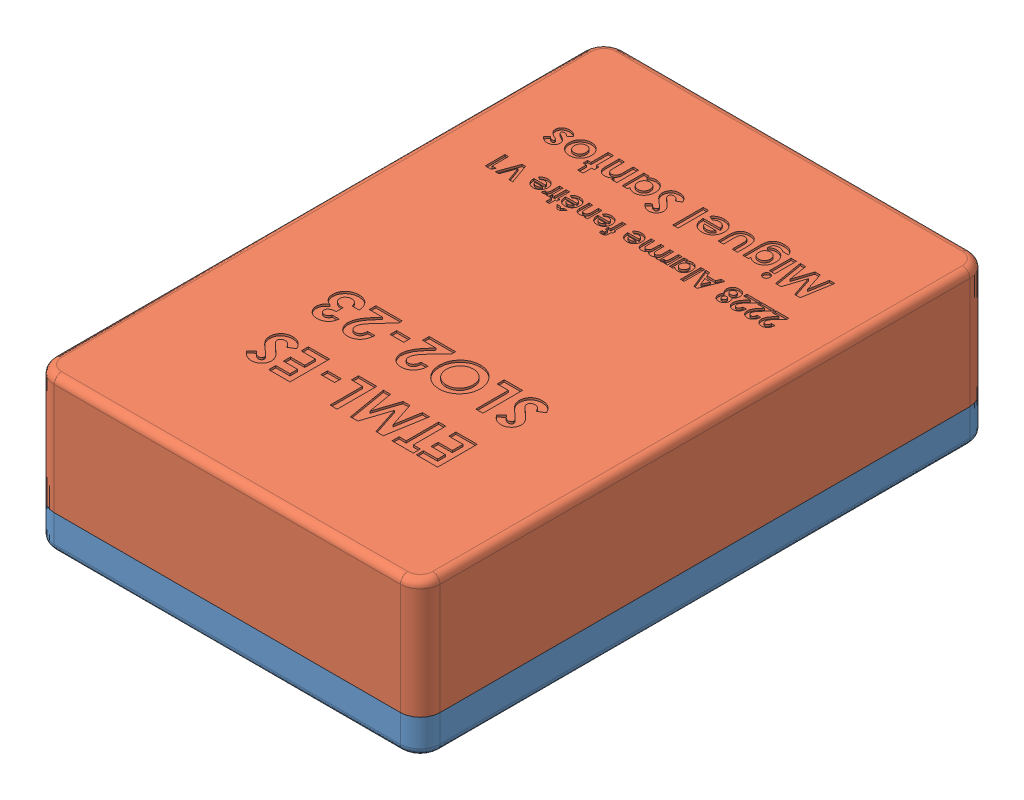
SolidWorks assembly 2228_Emetteur_Assembly, configuration Défaut. Lengths in mm.
Overall size (78 31 115.1).
221 component instances, 55 part files, 8 mates.
Components (placement in the parent):
- 2228_Emetteur_Bottom-1: 2228_Emetteur_Bottom [Défaut] at origin size (78 8.5 115.1)
- 2228_Emetteur_Top-1: 2228_Emetteur_Top [Défaut] at (0 31 0) x (-1 0 0) z (0 0 1) size (78 28 115.1)
- 22280A_AlarmeFenetre_Emetteur.step-1: 22280A_AlarmeFenetre_Emetteur.step [Défaut] at (30 7.1063 -64.5) x (-1 0 0) z (0 1 0) size (64.32 60 20.1)
  - Board.step-1: Board.step [Défaut] at origin size (60 60 1.61)
    - Open CASCADE STEP translator 6.8 1.1.1.step-1: Open CASCADE STEP translator 6.8 1.1.1.step [Défaut] at (0 0 -1.6063) size (60 60 1.61)
  - X3.step-1: X3.step [Défaut] at origin size (5.08 5.08 11.54)
    - 61300421121.step-1: 61300421121.step [Défaut] at (31.75 25 1.27) x (0 1 0) z (1 0 0) size (5.08 11.54 5.08)
      - Open CASCADE STEP translator 6.8 1.2.1.1.step-1: Open CASCADE STEP translator 6.8 1.2.1.1.step [Défaut] at origin size (5.08 2.54 5.08)
      - Open CASCADE STEP translator 6.8 1.2.1.2.step-1: Open CASCADE STEP translator 6.8 1.2.1.2.step [Défaut] at origin size (0.64 11.54 0.64)
      - Open CASCADE STEP translator 6.8 1.2.1.3.step-1: Open CASCADE STEP translator 6.8 1.2.1.3.step [Défaut] at origin size (0.64 11.54 0.64)
      - Open CASCADE STEP translator 6.8 1.2.1.4.step-1: Open CASCADE STEP translator 6.8 1.2.1.4.step [Défaut] at origin size (0.64 11.54 0.64)
      - Open CASCADE STEP translator 6.8 1.2.1.5.step-1: Open CASCADE STEP translator 6.8 1.2.1.5.step [Défaut] at origin size (0.64 11.54 0.64)
  - X5.step-1: X5.step [Défaut] at origin size (5.08 5.08 11.54)
    - 61300421121.step-1: 61300421121.step [Défaut] at (21.59 25 1.27) x (0 1 0) z (1 0 0) size (5.08 11.54 5.08)
      - Open CASCADE STEP translator 6.8 1.2.1.1.step-1: Open CASCADE STEP translator 6.8 1.2.1.1.step [Défaut] at origin size (5.08 2.54 5.08)
      - Open CASCADE STEP translator 6.8 1.2.1.2.step-1: Open CASCADE STEP translator 6.8 1.2.1.2.step [Défaut] at origin size (0.64 11.54 0.64)
      - Open CASCADE STEP translator 6.8 1.2.1.3.step-1: Open CASCADE STEP translator 6.8 1.2.1.3.step [Défaut] at origin size (0.64 11.54 0.64)
      - Open CASCADE STEP translator 6.8 1.2.1.4.step-1: Open CASCADE STEP translator 6.8 1.2.1.4.step [Défaut] at origin size (0.64 11.54 0.64)
      - Open CASCADE STEP translator 6.8 1.2.1.5.step-1: Open CASCADE STEP translator 6.8 1.2.1.5.step [Défaut] at origin size (0.64 11.54 0.64)
  - X4.step-1: X4.step [Défaut] at origin size (5.08 5.08 11.54)
    - 61300421121.step-1: 61300421121.step [Défaut] at (10.16 26.27 1.27) x (-1 0 0) z (0 1 0) size (5.08 11.54 5.08)
      - Open CASCADE STEP translator 6.8 1.2.1.1.step-1: Open CASCADE STEP translator 6.8 1.2.1.1.step [Défaut] at origin size (5.08 2.54 5.08)
      - Open CASCADE STEP translator 6.8 1.2.1.2.step-1: Open CASCADE STEP translator 6.8 1.2.1.2.step [Défaut] at origin size (0.64 11.54 0.64)
      - Open CASCADE STEP translator 6.8 1.2.1.3.step-1: Open CASCADE STEP translator 6.8 1.2.1.3.step [Défaut] at origin size (0.64 11.54 0.64)
      - Open CASCADE STEP translator 6.8 1.2.1.4.step-1: Open CASCADE STEP translator 6.8 1.2.1.4.step [Défaut] at origin size (0.64 11.54 0.64)
      - Open CASCADE STEP translator 6.8 1.2.1.5.step-1: Open CASCADE STEP translator 6.8 1.2.1.5.step [Défaut] at origin size (0.64 11.54 0.64)
  - X2.step-1: X2.step [Défaut] at origin size (5.08 5.08 11.54)
    - 61300421121.step-1: 61300421121.step [Défaut] at (39.37 25 1.27) x (0 -1 0) z (-1 0 0) size (5.08 11.54 5.08)
      - Open CASCADE STEP translator 6.8 1.2.1.1.step-1: Open CASCADE STEP translator 6.8 1.2.1.1.step [Défaut] at origin size (5.08 2.54 5.08)
      - Open CASCADE STEP translator 6.8 1.2.1.2.step-1: Open CASCADE STEP translator 6.8 1.2.1.2.step [Défaut] at origin size (0.64 11.54 0.64)
      - Open CASCADE STEP translator 6.8 1.2.1.3.step-1: Open CASCADE STEP translator 6.8 1.2.1.3.step [Défaut] at origin size (0.64 11.54 0.64)
      - Open CASCADE STEP translator 6.8 1.2.1.4.step-1: Open CASCADE STEP translator 6.8 1.2.1.4.step [Défaut] at origin size (0.64 11.54 0.64)
      - Open CASCADE STEP translator 6.8 1.2.1.5.step-1: Open CASCADE STEP translator 6.8 1.2.1.5.step [Défaut] at origin size (0.64 11.54 0.64)
  - X1.step-1: X1.step [Défaut] at origin size (2.54 5.08 11.54)
    - STEP-61300211121-rev1.step-1: STEP-61300211121-rev1.step [Défaut] at (11.9999 6.27 1.27) x (0 -1 0) z (-1 0 0) size (5.08 11.54 2.54)
      - 6130xx11121_PIN.step-1: 6130xx11121_PIN.step [Défaut] at (-1.27 1.5 0) x (1 0 0) z (0 -1 0) size (0.64 0.64 11.54)
      - 6130xx11121_PIN.step-2: 6130xx11121_PIN.step [Défaut] at (1.27 1.5 0) x (1 0 0) z (0 -1 0) size (0.64 0.64 11.54)
      - 61300211121.step-1: 61300211121.step [Défaut] at origin size (5.08 2.54 2.54)
  - VSTOR.step-1: VSTOR.step [Défaut] at origin size (3.81 2.03 2.29)
    - keystone-PN5019.step-1: keystone-PN5019.step [Défaut] at (56.9999 22.0009 0) x (1 0 0) z (0 -1 0) size (3.81 2.29 2.03)
  - VSEC.step-1: VSEC.step [Défaut] at origin size (3.81 2.03 2.29)
    - keystone-PN5019.step-1: keystone-PN5019.step [Défaut] at (57.0001 15.9991 0) x (-1 0 0) z (0 1 0) size (3.81 2.29 2.03)
  - VMUL.step-1: VMUL.step [Défaut] at origin size (3.81 2.03 2.29)
    - keystone-PN5019.step-1: keystone-PN5019.step [Défaut] at (3.0001 21.9991 0) x (-1 0 0) z (0 1 0) size (3.81 2.29 2.03)
  - VIN.step-1: VIN.step [Défaut] at origin size (3.81 2.03 2.29)
    - keystone-PN5019.step-1: keystone-PN5019.step [Défaut] at (2.9999 10.0009 0) x (1 0 0) z (0 -1 0) size (3.81 2.29 2.03)
  - VCC.step-1: VCC.step [Défaut] at origin size (3.81 2.03 2.29)
    - keystone-PN5019.step-1: keystone-PN5019.step [Défaut] at (3.0001 27.9991 0) x (-1 0 0) z (0 1 0) size (3.81 2.29 2.03)
  - U6.step-1: U6.step [Défaut] at origin size (46.04 19.26 18.6)
    - 61301011821.step-1: 61301011821.step [Défaut] at (1.27 49.62 0) x (1 0 0) z (0 0 1) size (25.9 2.5 11.6)
      - Body.step-1: Body.step [Défaut] at origin size (25.9 2.5 8.5)
      - LeadsArray.step-1: LeadsArray.step [Défaut] at origin size (23.46 0.6 4.8)
    - 61301011821.step-2: 61301011821.step [Défaut] at (1.27 34.38 0) x (1 0 0) z (0 0 1) size (25.9 2.5 11.6)
      - Body.step-1: Body.step [Défaut] at origin size (25.9 2.5 8.5)
      - LeadsArray.step-1: LeadsArray.step [Défaut] at origin size (23.46 0.6 4.8)
    - Conn_Wurth_Elektronik_61301011121_eec.step-1: Conn_Wurth_Elektronik_61301011121_eec.step [Défaut] at (12.7 49.62 10) x (1 0 0) z (0 1 0) size (25.4 11.74 4.02)
      - Package.step-1: Package.step [Défaut] at origin size (25.4 2.54 2.54)
      - Pins.step-1: Pins.step [Défaut] at origin size (23.5 11.74 0.64)
      - Logo.step-1: Logo.step [Défaut] at (12.7 -1.27 1.27) size (5.18 4.49 4.02)
    - Conn_Wurth_Elektronik_61301011121_eec.step-2: Conn_Wurth_Elektronik_61301011121_eec.step [Défaut] at (12.7 34.38 10) x (1 0 0) z (0 1 0) size (25.4 11.74 4.02)
      - Package.step-1: Package.step [Défaut] at origin size (25.4 2.54 2.54)
      - Pins.step-1: Pins.step [Défaut] at origin size (23.5 11.74 0.64)
      - Logo.step-1: Logo.step [Défaut] at (12.7 -1.27 1.27) size (5.18 4.49 4.02)
    - 400250.step-1: 400250.step [Défaut] at (-4.318 42 13) x (1 0 0) z (0 0 1) size (46.04 15.24 4.57)
  - U5.step-1: U5.step [Défaut] at origin size (2.51 2.92 1.12)
    - 5881998176.step-1: 5881998176.step [Défaut] at (30 56 0) x (-1 0 0) z (0 1 0) size (2.51 1.12 2.92)
  - U4.step-1: U4.step [Défaut] at origin size (2.8 2.9 1.45)
    - 5881997696.step-1: 5881997696.step [Défaut] at (15 16.5 0) x (-1 0 0) z (0 1 0) size (2.8 1.45 2.9)
  - U3.step-1: U3.step [Défaut] at origin size (6.1 4.99 1.77)
    - 5882000496.step-1: 5882000496.step [Défaut] at (48 16 0) x (-1 0 0) z (0 0 1) size (6.1 4.99 1.77)
  - U2.step-1: U2.step [Défaut] at origin size (6.1 4.99 1.77)
    - 5882000496.step-1: 5882000496.step [Défaut] at (48 25 0) x (-1 0 0) z (0 0 1) size (6.1 4.99 1.77)
  - U1.step-1: U1.step [Défaut] at origin size (3.76 3.76 1.4)
    - RGR20_2P05X2P05_TEX.step-1: RGR20_2P05X2P05_TEX.step [Défaut] at (30 11.5 0) x (1 0 0) z (0 0 1) size (3.76 3.76 1.4)
  - S1.step-1: S1.step [Défaut] at origin size (23 8 1.9)
    - Anysolar_KXOB25.step-1: Anysolar_KXOB25.step [Défaut] at (30 5 -1.6063) x (1 0 0) z (0 0 -1) size (7.2 6.59 0.1)
    - Anysolar_KXOB25-0.step-1: Anysolar_KXOB25-0.step [Défaut] at (30 5 -1.6063) x (1 0 0) z (0 0 -1) size (23 8 1.8)
    - Anysolar_KXOB25-1.step-1: Anysolar_KXOB25-1.step [Défaut] at (30 5 -1.6063) x (1 0 0) z (0 0 -1) size (7.2 6.59 0.1)
    - Anysolar_KXOB25-2.step-1: Anysolar_KXOB25-2.step [Défaut] at (30 5 -1.6063) x (1 0 0) z (0 0 -1) size (7.2 6.59 0.1)
  - R6.step-1: R6.step [Défaut] at origin size (2 1.25 0.51)
    - Resistor_0805_Text.step-1: Resistor_0805_Text.step [Défaut] at (35 49.62 0) x (1 0 0) z (0 0 1) size (2 1.25 0.51)
      - Pin1Body.step-1: Pin1Body.step [Défaut] at (0 0 0.01) size (0.37 1.25 0.5)
      - Pin2Body.step-1: Pin2Body.step [Défaut] at (0 0 0.01) size (0.37 1.25 0.5)
      - CeramicBody.step-1: CeramicBody.step [Défaut] at (0 0 0.01) size (1.93 1.25 0.43)
      - CoatingBody.step-1: CoatingBody.step [Défaut] at (0 0 0.01) size (1.33 1.25 0.03)
      - Text1Body.step-1: Text1Body.step [Défaut] at (0 0 0.01) size (0.25 0.4 0.01)
      - Text2Body.step-1: Text2Body.step [Défaut] at (0 0 0.01) size (0.25 0.4 0.01)
      - Text3Body.step-1: Text3Body.step [Défaut] at (0 0 0.01) size (0.25 0.4 0.01)
      - Text4Body.step-1: Text4Body.step [Défaut] at (0 0 0.01) size (0.25 0.4 0.01)
  - R5.step-1: R5.step [Défaut] at origin size (2 1.25 0.51)
    - Resistor_0805_Text.step-1: Resistor_0805_Text.step [Défaut] at (32.5 4 0) x (1 0 0) z (0 0 1) size (2 1.25 0.51)
      - Pin1Body.step-1: Pin1Body.step [Défaut] at (0 0 0.01) size (0.37 1.25 0.5)
      - Pin2Body.step-1: Pin2Body.step [Défaut] at (0 0 0.01) size (0.37 1.25 0.5)
      - CeramicBody.step-1: CeramicBody.step [Défaut] at (0 0 0.01) size (1.93 1.25 0.43)
      - CoatingBody.step-1: CoatingBody.step [Défaut] at (0 0 0.01) size (1.33 1.25 0.03)
      - Text1Body.step-1: Text1Body.step [Défaut] at (0 0 0.01) size (0.25 0.4 0.01)
      - Text2Body.step-1: Text2Body.step [Défaut] at (0 0 0.01) size (0.25 0.4 0.01)
      - Text3Body.step-1: Text3Body.step [Défaut] at (0 0 0.01) size (0.25 0.4 0.01)
      - Text4Body.step-1: Text4Body.step [Défaut] at (0 0 0.01) size (0.25 0.4 0.01)
  - R4.step-1: R4.step [Défaut] at origin size (2 1.25 0.51)
    - Resistor_0805_Text.step-1: Resistor_0805_Text.step [Défaut] at (34.5 6.5 0) x (1 0 0) z (0 0 1) size (2 1.25 0.51)
      - Pin1Body.step-1: Pin1Body.step [Défaut] at (0 0 0.01) size (0.37 1.25 0.5)
      - Pin2Body.step-1: Pin2Body.step [Défaut] at (0 0 0.01) size (0.37 1.25 0.5)
      - CeramicBody.step-1: CeramicBody.step [Défaut] at (0 0 0.01) size (1.93 1.25 0.43)
      - CoatingBody.step-1: CoatingBody.step [Défaut] at (0 0 0.01) size (1.33 1.25 0.03)
      - Text1Body.step-1: Text1Body.step [Défaut] at (0 0 0.01) size (0.25 0.4 0.01)
      - Text2Body.step-1: Text2Body.step [Défaut] at (0 0 0.01) size (0.25 0.4 0.01)
      - Text3Body.step-1: Text3Body.step [Défaut] at (0 0 0.01) size (0.25 0.4 0.01)
      - Text4Body.step-1: Text4Body.step [Défaut] at (0 0 0.01) size (0.25 0.4 0.01)
  - R3.step-1: R3.step [Défaut] at origin size (2 1.25 0.51)
    - Resistor_0805_Text.step-1: Resistor_0805_Text.step [Défaut] at (36.5 4 0) x (1 0 0) z (0 0 1) size (2 1.25 0.51)
      - Pin1Body.step-1: Pin1Body.step [Défaut] at (0 0 0.01) size (0.37 1.25 0.5)
      - Pin2Body.step-1: Pin2Body.step [Défaut] at (0 0 0.01) size (0.37 1.25 0.5)
      - CeramicBody.step-1: CeramicBody.step [Défaut] at (0 0 0.01) size (1.93 1.25 0.43)
      - CoatingBody.step-1: CoatingBody.step [Défaut] at (0 0 0.01) size (1.33 1.25 0.03)
      - Text1Body.step-1: Text1Body.step [Défaut] at (0 0 0.01) size (0.25 0.4 0.01)
      - Text2Body.step-1: Text2Body.step [Défaut] at (0 0 0.01) size (0.25 0.4 0.01)
      - Text3Body.step-1: Text3Body.step [Défaut] at (0 0 0.01) size (0.25 0.4 0.01)
      - Text4Body.step-1: Text4Body.step [Défaut] at (0 0 0.01) size (0.25 0.4 0.01)
  - R2.step-1: R2.step [Défaut] at origin size (2 1.25 0.51)
    - Resistor_0805_Text.step-1: Resistor_0805_Text.step [Défaut] at (30.5 6.5 0) x (-1 0 0) z (0 0 1) size (2 1.25 0.51)
      - Pin1Body.step-1: Pin1Body.step [Défaut] at (0 0 0.01) size (0.37 1.25 0.5)
      - Pin2Body.step-1: Pin2Body.step [Défaut] at (0 0 0.01) size (0.37 1.25 0.5)
      - CeramicBody.step-1: CeramicBody.step [Défaut] at (0 0 0.01) size (1.93 1.25 0.43)
      - CoatingBody.step-1: CoatingBody.step [Défaut] at (0 0 0.01) size (1.33 1.25 0.03)
      - Text1Body.step-1: Text1Body.step [Défaut] at (0 0 0.01) size (0.25 0.4 0.01)
      - Text2Body.step-1: Text2Body.step [Défaut] at (0 0 0.01) size (0.25 0.4 0.01)
      - Text3Body.step-1: Text3Body.step [Défaut] at (0 0 0.01) size (0.25 0.4 0.01)
      - Text4Body.step-1: Text4Body.step [Défaut] at (0 0 0.01) size (0.25 0.4 0.01)
  - R1.step-1: R1.step [Défaut] at origin size (2 1.25 0.51)
    - Resistor_0805_Text.step-1: Resistor_0805_Text.step [Défaut] at (28.5 4 0) x (-1 0 0) z (0 0 1) size (2 1.25 0.51)
      - Pin1Body.step-1: Pin1Body.step [Défaut] at (0 0 0.01) size (0.37 1.25 0.5)
      - Pin2Body.step-1: Pin2Body.step [Défaut] at (0 0 0.01) size (0.37 1.25 0.5)
      - CeramicBody.step-1: CeramicBody.step [Défaut] at (0 0 0.01) size (1.93 1.25 0.43)
      - CoatingBody.step-1: CoatingBody.step [Défaut] at (0 0 0.01) size (1.33 1.25 0.03)
      - Text1Body.step-1: Text1Body.step [Défaut] at (0 0 0.01) size (0.25 0.4 0.01)
      - Text2Body.step-1: Text2Body.step [Défaut] at (0 0 0.01) size (0.25 0.4 0.01)
      - Text3Body.step-1: Text3Body.step [Défaut] at (0 0 0.01) size (0.25 0.4 0.01)
      - Text4Body.step-1: Text4Body.step [Défaut] at (0 0 0.01) size (0.25 0.4 0.01)
  - Q1.step-1: Q1.step [Défaut] at origin size (1.2 1.2 0.55)
    - Trans_Rohm_RZM001P02T2L_eec.step-1: Trans_Rohm_RZM001P02T2L_eec.step [Défaut] at (35 52.5 0) x (0 1 0) z (0 0 1) size (1.2 1.2 0.55)
      - 1.step-1: 1.step [Défaut] at (0 0 0.05) x (0 -1 0) z (0 0 1) size (1.2 0.8 0.5)
      - 2.step-1: 2.step [Défaut] x (0 -1 0) z (0 0 1) size (1.02 1.2 0.13)
      - 3.step-1: 3.step [Défaut] at (0.0085 -0.0135 0.451) x (0 -1 0) z (0 0 1) size (0.31 0.18 0.11)
      - Notch.step-1: Notch.step [Défaut] at (-4.7119 3.8027 0.451) size (0.08 0.08 0.1)
  - L2.step-1: L2.step [Défaut] at origin size (2 1.25 0.6)
    - L_0805.step-1: L_0805.step [Défaut] at (10 13.5 0) x (-1 0 0) z (0 0 1) size (2 1.25 0.6)
      - Pin1.step-1: Pin1.step [Défaut] at origin size (0.62 1.25 0.6)
      - Pin2.step-1: Pin2.step [Défaut] at origin size (0.62 1.25 0.6)
      - CeramicBody-3.step-1: CeramicBody-3.step [Défaut] at origin size (1.8 1.23 0.58)
  - L1.step-1: L1.step [Défaut] at origin size (4.8 4.8 2.8)
    - 4828_74406043.step-1: 4828_74406043.step [Défaut] at (22.0529 15.7176 0) x (1 0 0) z (0 0 1) size (4.8 4.8 2.8)
      - Glue_L.step-1: Glue_L.step [Défaut] at (2.097 -0.9177 0.85) x (0 1 0) z (0 0 1) size (3.9 0.6 1.97)
      - Glue_R.step-1: Glue_R.step [Défaut] at (-1.203 -0.5177 0.85) x (0 1 0) z (0 0 1) size (3.9 0.6 1.95)
      - 4828_74406043-4.step-1: 4828_74406043-4.step [Défaut] at (0.447 -2.3677 0.001) size (3.26 2.73 2.5)
      - 4828_74406043-5.step-1: 4828_74406043-5.step [Défaut] at (0.447 -2.3677 0.001) size (3.9 3.3 2.8)
      - 4828_74406043_Housing.step-1: 4828_74406043_Housing.step [Défaut] at (0.447 -0.7177 0) size (4.8 4.8 2.8)
      - 4828_74406043_Pads.step-1: 4828_74406043_Pads.step [Défaut] at (-1.153 -0.7177 0) size (1.6 3.3 0.6)
      - 4828_74406043_Pads.step-2: 4828_74406043_Pads.step [Défaut] at (2.047 -0.7177 0) x (-1 0 0) z (0 0 1) size (1.6 3.3 0.6)
  - GND2.step-1: GND2.step [Défaut] at origin size (3.81 2.03 2.29)
    - keystone-PN5019.step-1: keystone-PN5019.step [Défaut] at (57.0001 9.9991 0) x (-1 0 0) z (0 1 0) size (3.81 2.29 2.03)
  - GND1.step-1: GND1.step [Défaut] at origin size (3.81 2.03 2.29)
    - keystone-PN5019.step-1: keystone-PN5019.step [Défaut] at (3.0001 15.9991 0) x (-1 0 0) z (0 1 0) size (3.81 2.29 2.03)
  - C9.step-1: C9.step [Défaut] at origin size (1.25 2 0.8)
    - Ceramic_Capacitor_0805_h32mil.step-1: Ceramic_Capacitor_0805_h32mil.step [Défaut] at (35 56 0) x (0 1 0) z (0 0 1) size (2 1.25 0.8)
      - Pin1-6.step-1: Pin1-6.step [Défaut] at origin size (0.62 1.25 0.8)
      - Pin2-7.step-1: Pin2-7.step [Défaut] at origin size (0.62 1.25 0.8)
      - CeramicBody-8.step-1: CeramicBody-8.step [Défaut] at origin size (1.8 1.23 0.78)
  - C8.step-1: C8.step [Défaut] at origin size (2 1.25 0.8)
    - Ceramic_Capacitor_0805_h32mil.step-1: Ceramic_Capacitor_0805_h32mil.step [Défaut] at (10 19.5 0) x (-1 0 0) z (0 0 1) size (2 1.25 0.8)
      - Pin1-6.step-1: Pin1-6.step [Défaut] at origin size (0.62 1.25 0.8)
      - Pin2-7.step-1: Pin2-7.step [Défaut] at origin size (0.62 1.25 0.8)
      - CeramicBody-8.step-1: CeramicBody-8.step [Défaut] at origin size (1.8 1.23 0.78)
  - C7.step-1: C7.step [Défaut] at origin size (2 1.25 0.8)
    - Ceramic_Capacitor_0805_h32mil.step-1: Ceramic_Capacitor_0805_h32mil.step [Défaut] at (10 16.5 0) x (1 0 0) z (0 0 1) size (2 1.25 0.8)
      - Pin1-6.step-1: Pin1-6.step [Défaut] at origin size (0.62 1.25 0.8)
      - Pin2-7.step-1: Pin2-7.step [Défaut] at origin size (0.62 1.25 0.8)
      - CeramicBody-8.step-1: CeramicBody-8.step [Défaut] at origin size (1.8 1.23 0.78)
  - C6.step-1: C6.step [Défaut] at origin size (2 1.25 0.8)
    - Ceramic_Capacitor_0805_h32mil.step-1: Ceramic_Capacitor_0805_h32mil.step [Défaut] at (30 16.5 0) x (1 0 0) z (0 0 1) size (2 1.25 0.8)
      - Pin1-6.step-1: Pin1-6.step [Défaut] at origin size (0.62 1.25 0.8)
      - Pin2-7.step-1: Pin2-7.step [Défaut] at origin size (0.62 1.25 0.8)
      - CeramicBody-8.step-1: CeramicBody-8.step [Défaut] at origin size (1.8 1.23 0.78)
  - C5.step-1: C5.step [Défaut] at origin size (2 1.25 0.8)
    - Ceramic_Capacitor_0805_h32mil.step-1: Ceramic_Capacitor_0805_h32mil.step [Défaut] at (30 19.5 0) x (1 0 0) z (0 0 1) size (2 1.25 0.8)
      - Pin1-6.step-1: Pin1-6.step [Défaut] at origin size (0.62 1.25 0.8)
      - Pin2-7.step-1: Pin2-7.step [Défaut] at origin size (0.62 1.25 0.8)
      - CeramicBody-8.step-1: CeramicBody-8.step [Défaut] at origin size (1.8 1.23 0.78)
  - C4.step-1: C4.step [Défaut] at origin size (2 1.25 0.8)
    - Ceramic_Capacitor_0805_h32mil.step-1: Ceramic_Capacitor_0805_h32mil.step [Défaut] at (48 10.5 0) x (-1 0 0) z (0 0 1) size (2 1.25 0.8)
      - Pin1-6.step-1: Pin1-6.step [Défaut] at origin size (0.62 1.25 0.8)
      - Pin2-7.step-1: Pin2-7.step [Défaut] at origin size (0.62 1.25 0.8)
      - CeramicBody-8.step-1: CeramicBody-8.step [Défaut] at origin size (1.8 1.23 0.78)
  - C3.step-1: C3.step [Défaut] at origin size (1.25 2 0.8)
    - Ceramic_Capacitor_0805_h32mil.step-1: Ceramic_Capacitor_0805_h32mil.step [Défaut] at (25 10 0) x (0 1 0) z (0 0 1) size (2 1.25 0.8)
      - Pin1-6.step-1: Pin1-6.step [Défaut] at origin size (0.62 1.25 0.8)
      - Pin2-7.step-1: Pin2-7.step [Défaut] at origin size (0.62 1.25 0.8)
      - CeramicBody-8.step-1: CeramicBody-8.step [Défaut] at origin size (1.8 1.23 0.78)
  - C2.step-1: C2.step [Défaut] at origin size (1.25 2 0.8)
    - Ceramic_Capacitor_0805_h32mil.step-1: Ceramic_Capacitor_0805_h32mil.step [Défaut] at (22.5 10 0) x (0 -1 0) z (0 0 1) size (2 1.25 0.8)
      - Pin1-6.step-1: Pin1-6.step [Défaut] at origin size (0.62 1.25 0.8)
      - Pin2-7.step-1: Pin2-7.step [Défaut] at origin size (0.62 1.25 0.8)
      - CeramicBody-8.step-1: CeramicBody-8.step [Défaut] at origin size (1.8 1.23 0.78)
  - C1.step-1: C1.step [Défaut] at origin size (1.25 2 0.8)
    - Ceramic_Capacitor_0805_h32mil.step-1: Ceramic_Capacitor_0805_h32mil.step [Défaut] at (20 10 0) x (0 -1 0) z (0 0 1) size (2 1.25 0.8)
      - Pin1-6.step-1: Pin1-6.step [Défaut] at origin size (0.62 1.25 0.8)
      - Pin2-7.step-1: Pin2-7.step [Défaut] at origin size (0.62 1.25 0.8)
      - CeramicBody-8.step-1: CeramicBody-8.step [Défaut] at origin size (1.8 1.23 0.78)
  - B2.step-1: B2.step [Défaut] at origin size (5.48 6.84 12.4)
    - Conn_W_rth_Elektronik_691210910002_eec.step-1: Conn_W_rth_Elektronik_691210910002_eec.step [Défaut] at (48 5 0) size (5.48 6.84 12.4)
      - 691210910002.step-1: 691210910002.step [Défaut] at (0 0 2.45) size (5.48 6.5 8.7)
      - 6912109100xx_CAGE.step-1: 6912109100xx_CAGE.step [Défaut] at (1.27 -0.175 2.65) size (2 3 3.9)
      - 6912109100xx_PIN.step-1: 6912109100xx_PIN.step [Défaut] at (1.27 0.195 1.8) x (-1 0 0) z (0 1 0) size (2.15 7.1 3.9)
      - 6912109100xx_VIS.step-1: 6912109100xx_VIS.step [Défaut] at (-1.27 -0.25 3.3) x (0 -1 0) z (0 0 1) size (2.1 2.1 4.45)
      - 6912109100xx_PIN.step-2: 6912109100xx_PIN.step [Défaut] at (-1.27 0.195 1.8) x (-1 0 0) z (0 1 0) size (2.15 7.1 3.9)
      - 6912109100xx_CAGE.step-2: 6912109100xx_CAGE.step [Défaut] at (-1.27 -0.175 2.65) size (2 3 3.9)
      - 6912109100xx_VIS.step-2: 6912109100xx_VIS.step [Défaut] at (1.27 -0.25 3.3) x (0 -1 0) z (0 0 1) size (2.1 2.1 4.45)
      - Logo.step-1: Logo.step [Défaut] at (2.74 -2.9 4.5) x (1 0 0) z (0 -0.972937 0.231072) size (5.18 4.49 4.02)
  - B1.step-1: B1.step [Défaut] at origin size (8.38 8 20.1)
    - 220uF_35V_electr_8_x16mm_-P.diameter_4mm.step-1: 220uF_35V_electr_8_x16mm_-P.diameter_4mm.step [Défaut] at (38.5 14.5 0) x (1 0 0) z (0 -1 0) size (8.38 20.1 8)
- keystone-PN2469.step-1: keystone-PN2469.step [Défaut] at (6.2774 15.2919 -91.2766) x (-1 0 0.000133) z (-0.000133 0 -1) size (69.29 27.34 37.92)
Mates (geometry in assembly coordinates):
- Coïncidente1: coincident anti-aligned: plane of 2228_Emetteur_Bottom_wPCB-1 through (0 7.05 0) normal (0 1 0); plane of 2228_Emetteur_Top-1 through (0 7.05 -57.55) normal (0 -1 0)
- Coïncidente2: coincident anti-aligned: line of 2228_Emetteur_Bottom_wPCB-1 through (-35 7.05 0) axis (1 0 0); line of 2228_Emetteur_Top-1 through (35 7.05 0) axis (-1 0 0)
- Coïncidente3: coincident anti-aligned: line of 2228_Emetteur_Bottom_wPCB-1 through (-39 7.05 -111.1) axis (0 0 1); line of 2228_Emetteur_Top-1 through (-39 7.05 -4) axis (0 0 -1)
- Coaxiale9: concentric anti-aligned: circle of 2228_Emetteur_Bottom_wPCB-1; circle of 22280A_AlarmeFenetre_Emetteur.step-1/Board.step-1/Open CASCADE STEP translator 6.8 1.1.1.step-1
- Coaxiale10: concentric aligned: cylinder of 2228_Emetteur_Bottom_wPCB-1 through (-26 1.5 -60.5) axis (0 1 0) radius 2; circle of 22280A_AlarmeFenetre_Emetteur.step-1/Board.step-1/Open CASCADE STEP translator 6.8 1.1.1.step-1
- Coïncidente6: coincident anti-aligned: plane of 2228_Emetteur_Bottom_wPCB-1 through (-26 5.5 -60.5) normal (0 1 0); plane of 22280A_AlarmeFenetre_Emetteur.step-1/Board.step-1/Open CASCADE STEP translator 6.8 1.1.1.step-1 through (26 5.5 -64.5) normal (0 -1 0)
- Coïncidente7: coincident anti-aligned: plane of 2228_Emetteur_Bottom_wPCB-1 through (0 5.5 0) normal (0 1 0); plane of keystone-PN2469.step-1 through (-26.8688 5.5 -102.2901) normal (0 -1 0)
- Coaxiale11: concentric anti-aligned: circle of 2228_Emetteur_Bottom_wPCB-1; cylinder of keystone-PN2469.step-1 through (-0.375 7.532 -90) axis (0 -1 0) radius 1.4986
